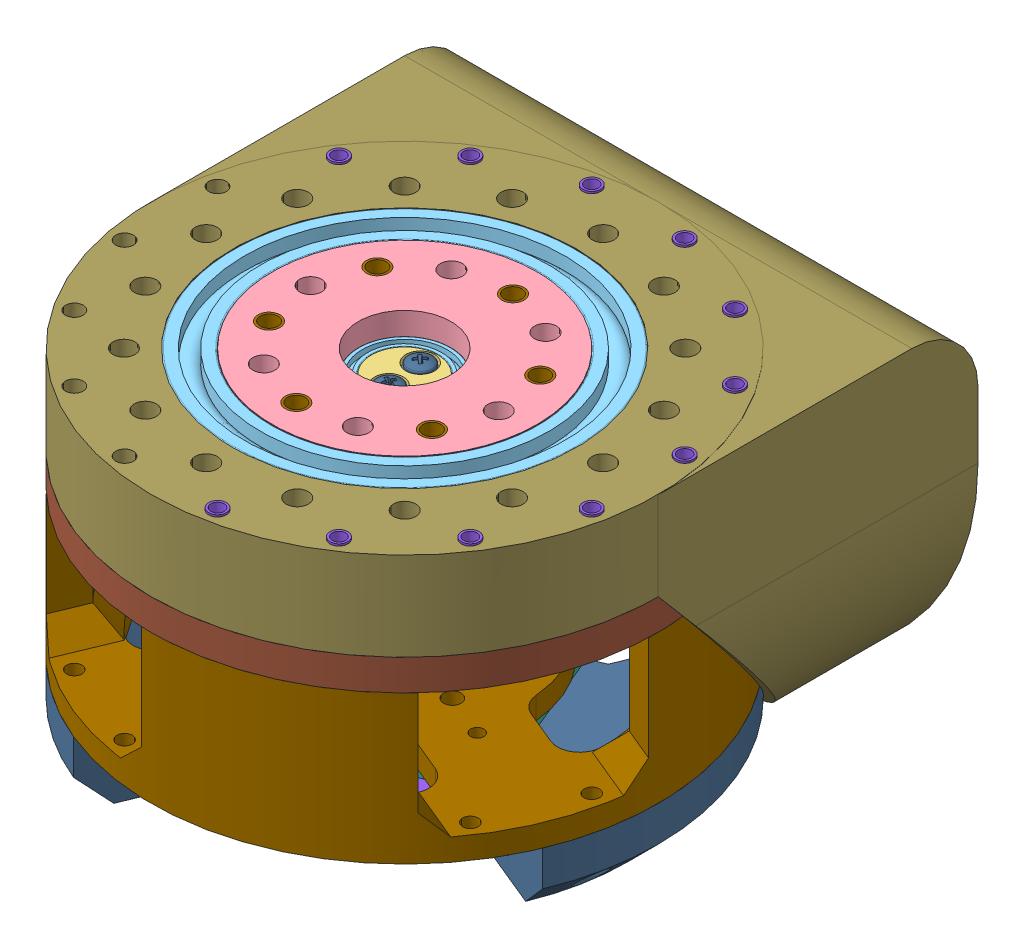
SolidWorks assembly Cycloidal_v3, configuration Default. Lengths in mm. (continued)
Components (placement in the parent): (continued)
- foc-motor-controller.step-1: foc-motor-controller.step [Default] at (47.267 33.7573 89.1587) x (-0.382683 0 -0.92388) z (0 -1 0) size (57.23 50 8.13) (continued)
  - C_1206_3216Metric.step-18: C_1206_3216Metric.step [Default] at (19.9 2.6 1.595) x (-0.707107 0.707107 0) z (0 0 1) size (3.2 1.6 1.6)
  - C_0603_1608Metric.step-27: C_0603_1608Metric.step [Default] at (13.4 -7.375 1.595) x (0 -1 0) z (0 0 1) size (1.6 0.8 0.8)
  - R_0603_1608Metric.step-25: R_0603_1608Metric.step [Default] at (8.7 -7.375 1.595) x (0 -1 0) z (0 0 1) size (1.6 0.8 0.45)
  - PQFN-8-EP_6x5mm_P1.27mm_Generic.step-1: PQFN-8-EP_6x5mm_P1.27mm_Generic.step [Default] at (4.9 14.4 -0.085) x (0 1 0) z (0 0 -1) size (6.15 5.15 1.09)
  - C_0805_2012Metric.step-3: C_0805_2012Metric.step [Default] at (-3 8.9 -0.085) x (0 1 0) z (0 0 -1) size (2 1.25 1.25)
  - C_0603_1608Metric.step-28: C_0603_1608Metric.step [Default] at (1.5 -4.3 -0.085) x (0 1 0) z (0 0 -1) size (1.6 0.8 0.8)
  - R_2512_6332Metric.step-1: R_2512_6332Metric.step [Default] at (2.1 8.6 -0.085) x (-1 0 0) z (0 0 -1) size (6.3 3.2 0.6)
  - C_0805_2012Metric.step-4: C_0805_2012Metric.step [Default] at (18.8 8.9 -0.085) x (0 1 0) z (0 0 -1) size (2 1.25 1.25)
  - C_0805_2012Metric.step-5: C_0805_2012Metric.step [Default] at (-5.2 8.901 -0.085) x (0 1 0) z (0 0 -1) size (2 1.25 1.25)
  - PQFN-8-EP_6x5mm_P1.27mm_Generic.step-2: PQFN-8-EP_6x5mm_P1.27mm_Generic.step [Default] at (16.9 14.6 -0.085) x (0 -1 0) z (0 0 -1) size (6.15 5.15 1.09)
  - PQFN-8-EP_6x5mm_P1.27mm_Generic.step-3: PQFN-8-EP_6x5mm_P1.27mm_Generic.step [Default] at (-1.1 14.6 -0.085) x (0 -1 0) z (0 0 -1) size (6.15 5.15 1.09)
  - R_0603_1608Metric.step-26: R_0603_1608Metric.step [Default] at (8.2 8.8 -0.085) x (0 1 0) z (0 0 -1) size (1.6 0.8 0.45)
  - R_2512_6332Metric.step-2: R_2512_6332Metric.step [Default] at (-10.3 8.601 -0.085) x (1 0 0) z (0 0 -1) size (6.3 3.2 0.6)
  - TSSOP-16_4.4x5mm_P0.65mm.step-1: TSSOP-16_4.4x5mm_P0.65mm.step [Default] at (0 0 -0.085) x (-1 0 0) z (0 0 -1) size (6.4 5 1.1)
  - C_0603_1608Metric.step-29: C_0603_1608Metric.step [Default] at (0 -4.25 -0.085) x (0 1 0) z (0 0 -1) size (1.6 0.8 0.8)
  - PQFN-8-EP_6x5mm_P1.27mm_Generic.step-4: PQFN-8-EP_6x5mm_P1.27mm_Generic.step [Default] at (10.9 14.4 -0.085) x (0 1 0) z (0 0 -1) size (6.15 5.15 1.09)
  - R_2512_6332Metric.step-3: R_2512_6332Metric.step [Default] at (13.7 8.6 -0.085) x (1 0 0) z (0 0 -1) size (6.3 3.2 0.6)
  - PQFN-8-EP_6x5mm_P1.27mm_Generic.step-5: PQFN-8-EP_6x5mm_P1.27mm_Generic.step [Default] at (-13.1 14.401 -0.085) x (0 1 0) z (0 0 -1) size (6.15 5.15 1.09)
  - C_0603_1608Metric.step-30: C_0603_1608Metric.step [Default] at (-1.5 -4.3 -0.085) x (0 -1 0) z (0 0 -1) size (1.6 0.8 0.8)
  - PQFN-8-EP_6x5mm_P1.27mm_Generic.step-6: PQFN-8-EP_6x5mm_P1.27mm_Generic.step [Default] at (-7.1 14.601 -0.085) x (0 -1 0) z (0 0 -1) size (6.15 5.15 1.09)
  - foc-motor-controller_PCB.step-1: foc-motor-controller_PCB.step [Default] at origin size (50 50 1.51)
- hex nut style 1 gradeab_iso-1: hex nut style 1 gradeab_iso [ISO - 4032 - M3 - W - N] at (35.6313 33.7573 117.2498) x (1 0 0) z (0 -1 0) size (5.5 6.35 2.4)
- Cycloidal_Discs_8308-1: Cycloidal_Discs_8308 [Default] at (-16.3285 42.227 57.9303) x (0.867922 0 -0.4967) z (0.4967 0 0.867922) size (79.25 5 79.73)
  - Cycloidal_Discs-1: Cycloidal_Discs [Default] at (38.3081 39.5303 58.0959) size (79.25 5 79.73)
  - radial ball bearing_68_iso-1: radial ball bearing_68_iso [ISO 15 RBB - 274 - 14,SI,NC,14_68] at (18.3896 43.2803 46.5959) x (0 1 0) z (0 0 1) size (2.5 7 7)
  - radial ball bearing_68_iso-2: radial ball bearing_68_iso [ISO 15 RBB - 274 - 14,SI,NC,14_68] at (38.3081 43.2803 81.0959) x (0 1 0) z (0 0 1) size (2.5 7 7)
  - radial ball bearing_68_iso-3: radial ball bearing_68_iso [ISO 15 RBB - 274 - 14,SI,NC,14_68] at (18.3896 43.2803 69.5959) x (0 1 0) z (0 0 1) size (2.5 7 7)
  - radial ball bearing_68_iso-4: radial ball bearing_68_iso [ISO 15 RBB - 274 - 14,SI,NC,14_68] at (38.3081 43.2803 35.0959) x (0 1 0) z (0 0 1) size (2.5 7 7)
  - radial ball bearing_68_iso-5: radial ball bearing_68_iso [ISO 15 RBB - 274 - 14,SI,NC,14_68] at (58.2267 43.2803 69.5959) x (0 1 0) z (0 0 1) size (2.5 7 7)
  - radial ball bearing_68_iso-6: radial ball bearing_68_iso [ISO 15 RBB - 274 - 14,SI,NC,14_68] at (58.2267 43.2803 46.5959) x (0 1 0) z (0 0 1) size (2.5 7 7)
- Cycloidal_Discs_8308-2: Cycloidal_Discs_8308 [Default] at (52.7572 37.227 19.5179) x (0.801823 0 0.597561) z (-0.597561 0 0.801823) size (79.25 5 79.73)
  - Cycloidal_Discs-1: Cycloidal_Discs [Default] at (38.3081 39.5303 58.0959) size (79.25 5 79.73)
  - radial ball bearing_68_iso-1: radial ball bearing_68_iso [ISO 15 RBB - 274 - 14,SI,NC,14_68] at (18.3896 43.2803 46.5959) x (0 1 0) z (0 0 1) size (2.5 7 7)
  - radial ball bearing_68_iso-2: radial ball bearing_68_iso [ISO 15 RBB - 274 - 14,SI,NC,14_68] at (38.3081 43.2803 81.0959) x (0 1 0) z (0 0 1) size (2.5 7 7)
  - radial ball bearing_68_iso-3: radial ball bearing_68_iso [ISO 15 RBB - 274 - 14,SI,NC,14_68] at (18.3896 43.2803 69.5959) x (0 1 0) z (0 0 1) size (2.5 7 7)
  - radial ball bearing_68_iso-4: radial ball bearing_68_iso [ISO 15 RBB - 274 - 14,SI,NC,14_68] at (38.3081 43.2803 35.0959) x (0 1 0) z (0 0 1) size (2.5 7 7)
  - radial ball bearing_68_iso-5: radial ball bearing_68_iso [ISO 15 RBB - 274 - 14,SI,NC,14_68] at (58.2267 43.2803 69.5959) x (0 1 0) z (0 0 1) size (2.5 7 7)
  - radial ball bearing_68_iso-6: radial ball bearing_68_iso [ISO 15 RBB - 274 - 14,SI,NC,14_68] at (58.2267 43.2803 46.5959) x (0 1 0) z (0 0 1) size (2.5 7 7)
- m6-1: m6 [Default] at (34.3944 92.633 108.219) x (0 0 -1) z (-1 0 0) size (6 16 6)
- Motor_Cover_v2-2: Motor_Cover_v2 [Default] at (47.267 36.1573 89.1587) x (-0.92388 0 -0.382683) z (0.382683 0 -0.92388) size (115 33.6 115)
- driver_cover-1: driver_cover [Default] at (47.267 36.1573 89.1587) x (-0.384295 0 -0.92321) z (-0.92321 0 0.384295) size (81.32 15 115)
- Base_plate_2-1: Base_plate_2 [Default] at (47.267 69.7573 89.1587) size (115 7 115)
- Cover_new-1: Cover_new [Default] at (47.267 86.8173 89.1587) size (115 87.56 130)
Mates (geometry in assembly coordinates):
- Coincident1: coincident anti-aligned: plane of motor-X83008S.stp-1/outrunner.stp-1 through (12.9806 69.7573 92.9922) normal (0 1 0); plane of Base_Plate-1 through (47.267 69.7573 89.1587) normal (0 -1 0)
- Concentric1: concentric anti-aligned: line of motor-X83008S.stp-1/outrunner.stp-1 through (31.863 64.2573 90.881) axis (0 1 0); cylinder of Base_Plate-1 through (31.863 76.7573 90.881) axis (0 -1 0) radius 1.5
- Concentric2: concentric anti-aligned: cylinder of motor-X83008S.stp-1/shaft.stp-1 through (47.267 69.7573 89.1587) axis (0 1 0) radius 1.5; line of Base_Plate-1 through (47.267 76.7573 89.1587) axis (0 -1 0)
- Coincident2: coincident anti-aligned: plane of Base_Plate-1 through (47.267 76.7573 89.1587) normal (0 1 0); plane of Eccentric_Shaft-1/Eccentric_Shaft_bot-1 through (48.7577 76.7573 88.992) normal (0 -1 0)
- Concentric75: concentric anti-aligned: cylinder of Output_Shaft-1 through (47.267 96.8173 89.1587) axis (0 -1 0) radius 30; cylinder of radial ball bearing_68_iso-39 through (47.267 71.1798 89.1587) axis (0 1 0) radius 30
- Concentric78: concentric anti-aligned: cylinder of Base_Plate-1 through (47.267 76.7573 89.1587) axis (0 -1 0) radius 20; cylinder of radial ball bearing_68_iso-40 through (47.267 52.6198 89.1587) axis (0 1 0) radius 20
- Concentric118: concentric anti-aligned: cylinder of Output_Shaft-1 through (37.1966 96.8173 68.4805) axis (0 -1 0) radius 2.5; cylinder of M4x6x5.5_brass_insert-1 through (37.1966 86.633 68.4805) axis (0 1 0) radius 2
- Concentric14021: concentric aligned: cylinder of Output_Shaft-1 through (70.21 96.8173 90.7765) axis (0 -1 0) radius 2.5; cylinder of M4x6x5.5_brass_insert-4 through (70.21 80.689 90.7765) axis (0 -1 0) radius 2.5
- Concentric14031: concentric aligned: cylinder of Output_Shaft-1 through (57.3374 96.8173 109.8369) axis (0 -1 0) radius 2.5; cylinder of M4x6x5.5_brass_insert-5 through (57.3374 80.689 109.8369) axis (0 -1 0) radius 2.5
- Concentric14041: concentric aligned: cylinder of Output_Shaft-1 through (34.3944 96.8173 108.219) axis (0 -1 0) radius 2.5; cylinder of M4x6x5.5_brass_insert-6 through (34.3944 80.689 108.219) axis (0 -1 0) radius 2.5
- Concentric14051: concentric aligned: cylinder of Output_Shaft-1 through (24.324 96.8173 87.5408) axis (0 -1 0) radius 2.5; cylinder of M4x6x5.5_brass_insert-7 through (24.324 80.689 87.5408) axis (0 -1 0) radius 2.5
- Concentric14061: concentric aligned: cylinder of Output_Shaft-1 through (48.8849 96.8173 66.2156) axis (0 -1 0) radius 2.5; cylinder of M4x6x5.5_brass_insert-8 through (48.8849 84.8733 66.2156) axis (0 -1 0) radius 2.5
- Concentric14071: concentric aligned: cylinder of Output_Shaft-1 through (28.2067 96.8173 76.286) axis (0 -1 0) radius 2.5; cylinder of M4x6x5.5_brass_insert-9 through (28.2067 84.8733 76.286) axis (0 -1 0) radius 2.5
- Concentric14081: concentric aligned: cylinder of Output_Shaft-1 through (26.5888 96.8173 99.2291) axis (0 -1 0) radius 2.5; cylinder of M4x6x5.5_brass_insert-10 through (26.5888 84.8733 99.2291) axis (0 -1 0) radius 2.5
- Concentric14091: concentric aligned: cylinder of Output_Shaft-1 through (45.6491 96.8173 112.1017) axis (0 -1 0) radius 2.5; cylinder of M4x6x5.5_brass_insert-11 through (45.6491 84.8733 112.1017) axis (0 -1 0) radius 2.5
- Concentric14111: concentric aligned: cylinder of Output_Shaft-1 through (66.3273 96.8173 102.0313) axis (0 -1 0) radius 2.5; cylinder of M4x6x5.5_brass_insert-13 through (66.3273 84.8733 102.0313) axis (0 -1 0) radius 2.5
- Concentric14121: concentric aligned: cylinder of Output_Shaft-1 through (67.9452 96.8173 79.0883) axis (0 -1 0) radius 2.5; cylinder of M4x6x5.5_brass_insert-14 through (67.9452 84.8733 79.0883) axis (0 -1 0) radius 2.5
- Concentric14131: concentric aligned: cylinder of Output_Shaft-1 through (60.1396 96.8173 70.0984) axis (0 -1 0) radius 2.5; cylinder of M4x6x5.5_brass_insert-15 through (60.1396 80.689 70.0984) axis (0 -1 0) radius 2.5
- Coincident1435: coincident aligned: plane of M4x6x5.5_brass_insert-1 through (35.332 92.633 70.1458) normal (0 1 0); plane of M4x6x5.5_brass_insert-15 through (60.1396 92.633 70.0984) normal (0 1 0)
- Coincident1436: coincident aligned: plane of M4x6x5.5_brass_insert-1 through (35.332 92.633 70.1458) normal (0 1 0); plane of M4x6x5.5_brass_insert-4 through (70.21 92.633 90.7765) normal (0 1 0)
- Coincident1437: coincident aligned: plane of M4x6x5.5_brass_insert-1 through (35.332 92.633 70.1458) normal (0 1 0); plane of M4x6x5.5_brass_insert-5 through (57.3374 92.633 109.8369) normal (0 1 0)
- Coincident1438: coincident aligned: plane of M4x6x5.5_brass_insert-1 through (35.332 92.633 70.1458) normal (0 1 0); plane of M4x6x5.5_brass_insert-6 through (34.3944 92.633 108.219) normal (0 1 0)
- Coincident1439: coincident aligned: plane of M4x6x5.5_brass_insert-1 through (35.332 92.633 70.1458) normal (0 1 0); plane of M4x6x5.5_brass_insert-7 through (24.324 92.633 87.5408) normal (0 1 0)
- Coincident1440: coincident aligned: plane of Output_Shaft-1 through (47.267 96.8173 89.1587) normal (0 1 0); plane of M4x6x5.5_brass_insert-9 through (28.2067 96.8173 76.286) normal (0 1 0)
- Coincident1441: coincident aligned: plane of Output_Shaft-1 through (47.267 96.8173 89.1587) normal (0 1 0); plane of M4x6x5.5_brass_insert-8 through (48.8849 96.8173 66.2156) normal (0 1 0)
- Coincident1442: coincident aligned: plane of Output_Shaft-1 through (47.267 96.8173 89.1587) normal (0 1 0); plane of M4x6x5.5_brass_insert-14 through (67.9452 96.8173 79.0883) normal (0 1 0)
- Coincident1443: coincident aligned: plane of Output_Shaft-1 through (47.267 96.8173 89.1587) normal (0 1 0); plane of M4x6x5.5_brass_insert-13 through (66.3273 96.8173 102.0313) normal (0 1 0)
- Coincident1444: coincident aligned: plane of Output_Shaft-1 through (47.267 96.8173 89.1587) normal (0 1 0); plane of M4x6x5.5_brass_insert-11 through (45.6491 96.8173 112.1017) normal (0 1 0)
- Coincident1445: coincident aligned: plane of Output_Shaft-1 through (47.267 96.8173 89.1587) normal (0 1 0); plane of M4x6x5.5_brass_insert-10 through (26.5888 96.8173 99.2291) normal (0 1 0)
- Concentric14151: concentric aligned: cylinder of m13_bearing-2/m6-1 through (64.4877 86.8573 130.7332) axis (0 1 0) radius 2; cylinder of M4x6x5.5_brass_insert-20 through (64.4877 86.8573 130.7332) axis (0 1 0) radius 2
- Concentric14161: concentric aligned: cylinder of m13_bearing-11/m6-1 through (47.267 86.8573 134.1587) axis (0 1 0) radius 2; cylinder of M4x6x5.5_brass_insert-21 through (47.267 86.8573 134.1587) axis (0 1 0) radius 2
- Concentric14171: concentric aligned: cylinder of m13_bearing-1/m6-1 through (15.4472 86.8573 57.3389) axis (0 1 0) radius 2; cylinder of M4x6x5.5_brass_insert-22 through (15.4472 86.8573 57.3389) axis (0 1 0) radius 2
- Concentric14181: concentric aligned: cylinder of m13_bearing-6/m6-1 through (30.0462 86.8573 47.5841) axis (0 1 0) radius 2; cylinder of M4x6x5.5_brass_insert-23 through (30.0462 86.8573 47.5841) axis (0 1 0) radius 2
- Concentric14191: concentric aligned: cylinder of m13_bearing-12/m6-1 through (79.0868 86.8573 120.9785) axis (0 1 0) radius 2; cylinder of M4x6x5.5_brass_insert-24 through (79.0868 98.8014 120.9785) axis (0 1 0) radius 2.3
- Concentric14201: concentric aligned: cylinder of m13_bearing-5/m6-1 through (88.8416 86.8573 106.3794) axis (0 1 0) radius 2; cylinder of M4x6x5.5_brass_insert-25 through (88.8416 86.8573 106.3794) axis (0 1 0) radius 2
- Concentric14211: concentric aligned: cylinder of m13_bearing-4/m6-1 through (92.267 86.7573 89.1587) axis (0 1 0) radius 2; cylinder of M4x6x5.5_brass_insert-26 through (92.267 86.8573 89.1587) axis (0 1 0) radius 2
- Concentric14221: concentric aligned: cylinder of m13_bearing-9/m6-1 through (88.8416 86.8573 71.9379) axis (0 1 0) radius 2; cylinder of M4x6x5.5_brass_insert-27 through (88.8416 86.8573 71.9379) axis (0 1 0) radius 2
- Concentric14241: concentric aligned: cylinder of m13_bearing-7/m6-1 through (64.4877 86.8573 47.5841) axis (0 1 0) radius 2; cylinder of M4x6x5.5_brass_insert-29 through (64.4877 86.8573 47.5841) axis (0 1 0) radius 2
- Concentric14251: concentric aligned: cylinder of m13_bearing-3/m6-1 through (47.267 86.8573 44.1587) axis (0 1 0) radius 2; cylinder of M4x6x5.5_brass_insert-31 through (47.267 86.8573 44.1587) axis (0 1 0) radius 2
- Coincident1447: coincident anti-aligned: plane of m13_bearing-2/m6-1 through (64.4877 86.8573 130.7332) normal (0 1 0); plane of M4x6x5.5_brass_insert-20 through (64.4877 86.8573 130.7332) normal (0 -1 0)
- Coincident1458: coincident aligned: plane of M4x6x5.5_brass_insert-20 through (62.6232 92.8573 132.3986) normal (0 1 0); plane of M4x6x5.5_brass_insert-21 through (45.4024 92.8573 135.824) normal (0 1 0)
- Coincident1459: coincident aligned: plane of M4x6x5.5_brass_insert-20 through (62.6232 92.8573 132.3986) normal (0 1 0); plane of M4x6x5.5_brass_insert-22 through (17.0054 92.8573 59.2938) normal (0 1 0)
- Coincident1460: coincident aligned: plane of M4x6x5.5_brass_insert-20 through (62.6232 92.8573 132.3986) normal (0 1 0); plane of M4x6x5.5_brass_insert-23 through (31.6045 92.8573 49.5391) normal (0 1 0)
- Coincident1461: coincident aligned: plane of M4x6x5.5_brass_insert-20 through (62.6232 92.8573 132.3986) normal (0 1 0); plane of M4x6x5.5_brass_insert-31 through (46.7161 92.8573 46.5972) normal (0 1 0)
- Coincident1462: coincident aligned: plane of M4x6x5.5_brass_insert-20 through (62.6232 92.8573 132.3986) normal (0 1 0); plane of M4x6x5.5_brass_insert-29 through (64.1304 92.8573 50.0584) normal (0 1 0)
- Coincident1463: coincident aligned: plane of M4x6x5.5_brass_insert-20 through (62.6232 92.8573 132.3986) normal (0 1 0); plane of M4x6x5.5_brass_insert-28 through (79.0868 92.8573 57.3389) normal (0 1 0)
- Coincident1464: coincident aligned: plane of M4x6x5.5_brass_insert-20 through (62.6232 92.8573 132.3986) normal (0 1 0); plane of M4x6x5.5_brass_insert-27 through (86.977 92.8573 73.6032) normal (0 1 0)
- Coincident1465: coincident aligned: plane of M4x6x5.5_brass_insert-20 through (62.6232 92.8573 132.3986) normal (0 1 0); plane of M4x6x5.5_brass_insert-26 through (90.4024 92.8573 90.824) normal (0 1 0)
- Coincident1466: coincident aligned: plane of M4x6x5.5_brass_insert-20 through (62.6232 92.8573 132.3986) normal (0 1 0); plane of M4x6x5.5_brass_insert-25 through (86.977 92.8573 108.0448) normal (0 1 0)
- Coincident1467: coincident aligned: plane of M4x6x5.5_brass_insert-20 through (62.6232 92.8573 132.3986) normal (0 1 0); plane of M4x6x5.5_brass_insert-24 through (80.4417 92.8573 123.0795) normal (0 1 0)
- Concentric1426: concentric aligned: cylinder of pan cross head_am-1 through (46.8225 118.0573 85.1834) axis (0 1 0) radius 1.5; line of Eccentric_Shaft-1/Eccentric_Shaft_top-1 through (46.8225 90.2573 85.1834) axis (0 1 0)
- Coincident1468: coincident anti-aligned: plane of Eccentric_Shaft-1/Eccentric_Shaft_top-1 through (47.7115 90.2573 93.1339) normal (0 1 0); plane of pan cross head_am-1 through (47.8167 90.2573 84.0602) normal (0 -1 0)
- Concentric14281: concentric aligned: cylinder of pan cross head_am-3 through (47.7115 118.0573 93.1339) axis (0 1 0) radius 2.8; cylinder of Eccentric_Shaft-1/Eccentric_Shaft_top-1 through (47.7115 86.7573 93.1339) axis (0 1 0) radius 1.5
- Coincident14701: coincident anti-aligned: plane of Eccentric_Shaft-1/Eccentric_Shaft_top-1 through (46.8225 90.2573 85.1834) normal (0 1 0); plane of pan cross head_am-3 through (48.2219 90.2573 91.7234) normal (0 -1 0)
- Concentric1437: concentric anti-aligned: cylinder of Base_Plate-1 through (46.8225 76.7573 85.1834) axis (0 -1 0) radius 2; cylinder of M3x4x4.2_brass_insert-22 through (46.8225 74.6594 85.1834) axis (0 1 0) radius 1.5
- Coincident1479: coincident aligned: plane of Base_Plate-1 through (47.267 69.7573 89.1587) normal (0 -1 0); plane of M3x4x4.2_brass_insert-22 through (48.2994 69.7573 84.921) normal (0 -1 0)
- Concentric1438: concentric anti-aligned: cylinder of Base_Plate-1 through (47.7115 76.7573 93.1339) axis (0 -1 0) radius 2; cylinder of M3x4x4.2_brass_insert-23 through (47.7115 74.6594 93.1339) axis (0 1 0) radius 1.5
- Coincident1480: coincident aligned: plane of Base_Plate-1 through (47.267 69.7573 89.1587) normal (0 -1 0); plane of M3x4x4.2_brass_insert-23 through (49.1884 69.7573 92.8717) normal (0 -1 0)
- Concentric1439: concentric anti-aligned: cylinder of Base_Plate-1 through (48.9893 76.7573 104.5627) axis (0 -1 0) radius 1.5; cylinder of pan cross head_am-4 through (48.9893 103.0573 104.5627) axis (0 1 0) radius 1.5
- Coincident1481: coincident anti-aligned: plane of Base_Plate-1 through (48.9893 75.2573 104.5627) normal (0 1 0); plane of pan cross head_am-4 through (50.4893 75.2573 104.5627) normal (0 -1 0)
- Concentric14401: concentric anti-aligned: cylinder of Base_Plate-1 through (45.5447 76.7573 73.7547) axis (0 -1 0) radius 1.5; cylinder of pan cross head_am-5 through (45.5447 103.0573 73.7547) axis (0 1 0) radius 2.8
- Coincident14821: coincident anti-aligned: plane of Base_Plate-1 through (45.5447 75.2573 73.7547) normal (0 1 0); plane of pan cross head_am-5 through (47.0447 75.2573 73.7547) normal (0 -1 0)
- GearMate1: gear = 10 : 1 mm: cylinder of Eccentric_Shaft-1/Eccentric_Shaft_top-1 through (47.267 91.7573 89.1587) axis (0 -1 0) radius 7.5; cylinder of Output_Shaft-1 through (47.267 96.8173 89.1587) axis (0 -1 0) radius 10.5
- Concentric1445021: concentric anti-aligned: cylinder of Base_Plate-1 through (62.671 76.7573 87.4364) axis (0 -1 0) radius 1.5; cylinder of pan cross head_am-6 through (62.671 103.0573 87.4364) axis (0 1 0) radius 2.8
- Coincident1486621: coincident anti-aligned: plane of Base_Plate-1 through (62.671 75.2573 87.4364) normal (0 1 0); plane of pan cross head_am-6 through (64.171 75.2573 87.4364) normal (0 -1 0)
- Concentric1445031: concentric anti-aligned: cylinder of Base_Plate-1 through (31.863 76.7573 90.881) axis (0 -1 0) radius 1.5; cylinder of pan cross head_am-7 through (31.863 103.0573 90.881) axis (0 1 0) radius 2.8
- Coincident1486631: coincident anti-aligned: plane of Base_Plate-1 through (31.863 75.2573 90.881) normal (0 1 0); plane of pan cross head_am-7 through (33.363 75.2573 90.881) normal (0 -1 0)
- Concentric1445035: concentric anti-aligned: cylinder of Eccentric_Shaft-1/Eccentric_Shaft_bot-1 through (48.7577 81.7573 88.992) axis (0 -1 0) radius 7.5; cylinder of radial ball bearing_68_iso-46 through (48.7577 59.1198 88.992) axis (0 1 0) radius 7.5
- Coincident1486648: coincident aligned: plane of Eccentric_Shaft-1/Eccentric_Shaft_bot-1 through (48.7577 81.7573 88.992) normal (0 1 0); plane of radial ball bearing_68_iso-46 through (41.0577 81.7573 88.9934) normal (0 1 0)
- Concentric1445036: concentric anti-aligned: cylinder of Eccentric_Shaft-1/Eccentric_Shaft_bot-2 through (45.7763 86.7573 89.3253) axis (0 -1 0) radius 7.5; cylinder of radial ball bearing_68_iso-44 through (45.7763 64.1198 89.3253) axis (0 1 0) radius 7.5
- Coincident1486649: coincident aligned: plane of Eccentric_Shaft-1/Eccentric_Shaft_bot-2 through (45.7763 82.7573 89.3253) normal (0 1 0); circle of radial ball bearing_68_iso-44
- Concentric1445037: concentric anti-aligned: cylinder of Eccentric_Shaft-1/Eccentric_Shaft_top-1 through (47.267 91.7573 89.1587) axis (0 -1 0) radius 7.5; cylinder of radial ball bearing_68_iso-45 through (47.267 69.1198 89.1587) axis (0 1 0) radius 7.5
- Concentric1445038: concentric anti-aligned: cylinder of Base_Plate-1 through (47.267 76.7573 89.1587) axis (0 -1 0) radius 20; cylinder of radial ball bearing_68_iso-40 through (47.267 52.6198 89.1587) axis (0 1 0) radius 20
- Coincident1486655: coincident anti-aligned: plane of Eccentric_Shaft-1/Eccentric_Shaft_top-1 through (47.267 87.7573 89.1587) normal (0 1 0); plane of radial ball bearing_68_iso-45 through (47.5372 87.7573 97.5543) normal (0 -1 0)
- Concentric1445042: concentric anti-aligned: cylinder of Base_Plate-1 through (47.7115 76.7573 93.1339) axis (0 -1 0) radius 2; cylinder of Eccentric_Shaft-1/Eccentric_Shaft_bot-1 through (47.7115 76.7573 93.1339) axis (0 1 0) radius 1.5
- Concentric1445043: concentric aligned: cylinder of Eccentric_Shaft-1/Eccentric_Shaft_bot-1 through (46.8225 76.7573 85.1834) axis (0 1 0) radius 1.5; cylinder of M3x4x4.2_brass_insert-22 through (46.8225 74.6594 85.1834) axis (0 1 0) radius 1.5
- Concentric1445052: concentric aligned: circle of m13_bearing-31/m6-1; cylinder of M4x6x5.5_brass_insert-47 through (5.6924 92.8573 71.9379) axis (0 -1 0) radius 2
- Concentric1445056: concentric aligned: circle of m13_bearing-32/m6-1; cylinder of M4x6x5.5_brass_insert-48 through (2.267 92.8573 89.1587) axis (0 -1 0) radius 2
- Coincident1486681: coincident anti-aligned: plane of m13_bearing-1/m6-1 through (15.4472 92.8573 57.3389) normal (0 1 0); circle of M4x6x5.5_brass_insert-47
- Concentric1445063: concentric aligned: cylinder of m13_bearing-34/m6-1 through (30.0462 87.0073 130.7332) axis (0 1 0) radius 2; cylinder of M4x6x5.5_brass_insert-51 through (30.0462 87.0073 130.7332) axis (0 1 0) radius 2
- Coincident1486686: coincident aligned: plane of m13_bearing-36/m6-1 through (5.6924 93.0073 106.3794) normal (0 1 0); circle of M4x6x5.5_brass_insert-49
- Coincident1486687: coincident anti-aligned: plane of m13_bearing-32/m6-1 through (2.267 92.8573 89.1587) normal (0 1 0); circle of M4x6x5.5_brass_insert-48
- Coincident1486688: coincident aligned: plane of m13_bearing-35/m6-1 through (15.4472 92.8573 120.9785) normal (0 1 0); circle of M4x6x5.5_brass_insert-50
- Coincident1486690: coincident aligned: plane of m13_bearing-34/m6-1 through (30.0462 93.0073 130.7332) normal (0 1 0); circle of M4x6x5.5_brass_insert-51
- Coincident1486692: coincident anti-aligned: plane of foc-motor-controller.step-1/foc-motor-controller_PCB.step-1 through (47.267 33.7573 89.1587) normal (0 1 0); plane of hex nut style 1 gradeab_iso-1 through (35.6313 33.7573 120.4252) normal (0 -1 0)
- Concentric14450545: concentric anti-aligned: cylinder of radial ball bearing_68_iso-46 through (48.7577 59.1198 88.992) axis (0 1 0) radius 10.5; cylinder of Cycloidal_Discs_8308-2/Cycloidal_Discs-1 through (48.7577 81.7573 88.992) axis (0 -1 0) radius 10.5
- Coincident1486693: coincident aligned: plane of radial ball bearing_68_iso-46 through (38.4577 81.7573 88.9938) normal (0 1 0); plane of Cycloidal_Discs_8308-2/Cycloidal_Discs-1 through (71.8151 81.7573 58.3329) normal (0 1 0)
- Concentric14450546: concentric anti-aligned: cylinder of radial ball bearing_68_iso-44 through (45.7763 64.1198 89.3253) axis (0 1 0) radius 10.5; cylinder of Cycloidal_Discs_8308-1/Cycloidal_Discs-1 through (45.7763 86.7573 89.3253) axis (0 -1 0) radius 10.5
- Coincident1486694: coincident aligned: plane of radial ball bearing_68_iso-44 through (52.9778 86.7573 81.9613) normal (0 1 0); plane of Cycloidal_Discs_8308-1/Cycloidal_Discs-1 through (26.8674 86.7573 55.9476) normal (0 1 0)
- Concentric14450547: concentric anti-aligned: cylinder of M4x6x5.5_brass_insert-6 through (34.3944 92.633 108.219) axis (0 -1 0) radius 2; cylinder of m6-1 through (34.3944 86.633 108.219) axis (0 1 0) radius 2
- Coincident1486695: coincident anti-aligned: circle of M4x6x5.5_brass_insert-6; plane of m6-1 through (34.3944 86.633 108.219) normal (0 1 0)
- Tangent1: tangent aligned: cylinder of Cycloidal_Discs_8308-1/radial ball bearing_68_iso-3 through (34.2006 64.8698 109.2) axis (0 1 0) radius 2; cylinder of m6-1 through (34.3944 76.633 108.219) axis (0 1 0) radius 3
- Tangent3: tangent aligned: cylinder of Cycloidal_Discs_8308-2/radial ball bearing_68_iso-2 through (35.0138 59.8698 107.4339) axis (0 1 0) radius 2; cylinder of m6-1 through (34.3944 76.633 108.219) axis (0 1 0) radius 3
- Concentric14450559: concentric anti-aligned: cylinder of foc-motor-controller.step-1/foc-motor-controller_PCB.step-1 through (58.9027 33.8033 61.0676) axis (0 1 0) radius 1.6; cylinder of Motor_Cover_v2-2 through (58.9027 86.1573 61.0676) axis (0 -1 0) radius 1.5
- Concentric14450560: concentric anti-aligned: circle of foc-motor-controller.step-1/foc-motor-controller_PCB.step-1; cylinder of Motor_Cover_v2-2 through (35.6313 86.1573 117.2498) axis (0 -1 0) radius 1.5
- Coincident1486699: coincident anti-aligned: line of foc-motor-controller.step-1/foc-motor-controller_PCB.step-1 through (35.6313 32.2473 117.2498) axis (0 1 0); line of hex nut style 1 gradeab_iso-1 through (35.6313 35.9569 117.2498) axis (0 -1 0)
- Coincident1486700: coincident aligned: circle of hex nut style 1 gradeab_iso-1; plane of Motor_Cover_v2-2 through (47.267 36.1573 89.1587) normal (0 -1 0)
- Concentric14450561: concentric anti-aligned: cylinder of Motor_Cover_v2-2 through (47.267 69.7573 89.1587) axis (0 -1 0) radius 57.5; cylinder of driver_cover-1 through (47.267 21.1573 89.1587) axis (0 1 0) radius 57.5
- Coincident1486701: coincident anti-aligned: plane of Motor_Cover_v2-2 through (47.267 36.1573 89.1587) normal (0 -1 0); plane of driver_cover-1 through (47.267 36.1573 89.1587) normal (0 1 0)
- Concentric14450565: concentric aligned: cylinder of m13_bearing-36/m6-1 through (5.6924 87.0073 106.3794) axis (0 1 0) radius 2; cylinder of M4x6x5.5_brass_insert-49 through (5.6924 87.0073 106.3794) axis (0 1 0) radius 2
- Concentric14450566: concentric aligned: cylinder of Motor_Cover_v2-2 through (92.1663 86.1573 59.1579) axis (0 -1 0) radius 1.75; cylinder of driver_cover-1 through (92.1663 36.1573 59.1579) axis (0 -1 0) radius 1.75
- Concentric14450569: concentric anti-aligned: cylinder of Base_Plate-1 through (47.267 76.7573 89.1587) axis (0 -1 0) radius 20; cylinder of radial ball bearing_68_iso-40 through (47.267 52.6198 89.1587) axis (0 1 0) radius 20
- Concentric14450570: concentric aligned: cylinder of Motor_Cover_v2-2 through (47.267 69.7573 89.1587) axis (0 -1 0) radius 57.5; cylinder of Base_plate_2-1 through (47.267 76.7573 89.1587) axis (0 -1 0) radius 57.5
- Concentric14450571: concentric anti-aligned: cylinder of radial ball bearing_68_iso-40 through (47.267 52.6198 89.1587) axis (0 1 0) radius 26; cylinder of Base_plate_2-1 through (47.267 76.7573 89.1587) axis (0 -1 0) radius 57.5
- Coincident1486702: coincident anti-aligned: plane of Motor_Cover_v2-2 through (47.267 69.7573 89.1587) normal (0 1 0); plane of Base_plate_2-1 through (47.267 69.7573 89.1587) normal (0 -1 0)
- Concentric14450572: concentric anti-aligned: cylinder of m13_bearing-5/radial ball bearing_68_iso-1 through (88.8416 99.9948 106.3794) axis (0 -1 0) radius 6.5; circle of Base_plate_2-1
- Concentric14450573: concentric anti-aligned: cylinder of radial ball bearing_68_iso-39 through (47.267 71.1798 89.1587) axis (0 1 0) radius 39; cylinder of Base_plate_2-1 through (47.267 76.7573 89.1587) axis (0 -1 0) radius 57.5
- Coincident1486703: coincident aligned: plane of Output_Shaft-1 through (47.267 96.8173 89.1587) normal (0 1 0); plane of radial ball bearing_68_iso-39 through (8.7841 96.8173 93.2526) normal (0 1 0)
- Coincident1486704: coincident anti-aligned: plane of Cycloidal_Discs_8308-2/Cycloidal_Discs-1 through (71.8151 76.7573 58.3329) normal (0 -1 0); plane of Base_plate_2-1 through (47.267 76.7573 89.1587) normal (0 1 0)
- Concentric14450574: concentric aligned: cylinder of Base_plate_2-1 through (47.267 76.7573 89.1587) axis (0 -1 0) radius 57.5; cylinder of Cover_new-1 through (47.267 96.8173 89.1587) axis (0 -1 0) radius 57.5
- Coincident1486705: coincident aligned: plane of Output_Shaft-1 through (47.267 96.8173 89.1587) normal (0 1 0); plane of Cover_new-1 through (47.267 96.8173 89.1587) normal (0 1 0)
- Concentric14450576: concentric anti-aligned: cylinder of m13_bearing-4/radial ball bearing_68_iso-2 through (92.267 104.8948 89.1587) axis (0 -1 0) radius 6.5; cylinder of Cover_new-1 through (92.267 76.7573 89.1587) axis (0 1 0) radius 7
- Concentric14450577: concentric anti-aligned: cylinder of m13_bearing-4/radial ball bearing_68_iso-2 through (92.267 104.8948 89.1587) axis (0 -1 0) radius 6.5; cylinder of Base_plate_2-1 through (92.267 75.7573 89.1587) axis (0 1 0) radius 5
- Coincident1486706: coincident anti-aligned: plane of m13_bearing-4/m6-1 through (92.267 76.7573 89.1587) normal (0 -1 0); plane of Base_plate_2-1 through (47.267 76.7573 89.1587) normal (0 1 0)
- Coincident1486707: coincident anti-aligned: plane of Base_plate_2-1 through (47.267 76.7573 89.1587) normal (0 1 0); plane of Cover_new-1 through (47.267 76.7573 89.1587) normal (0 -1 0)
- Concentric14450578: concentric aligned: cylinder of driver_cover-1 through (-5.6954 36.1573 99.6935) axis (0 -1 0) radius 1.75; cylinder of Base_plate_2-1 through (-5.6954 76.7573 99.6935) axis (0 -1 0) radius 1.75
